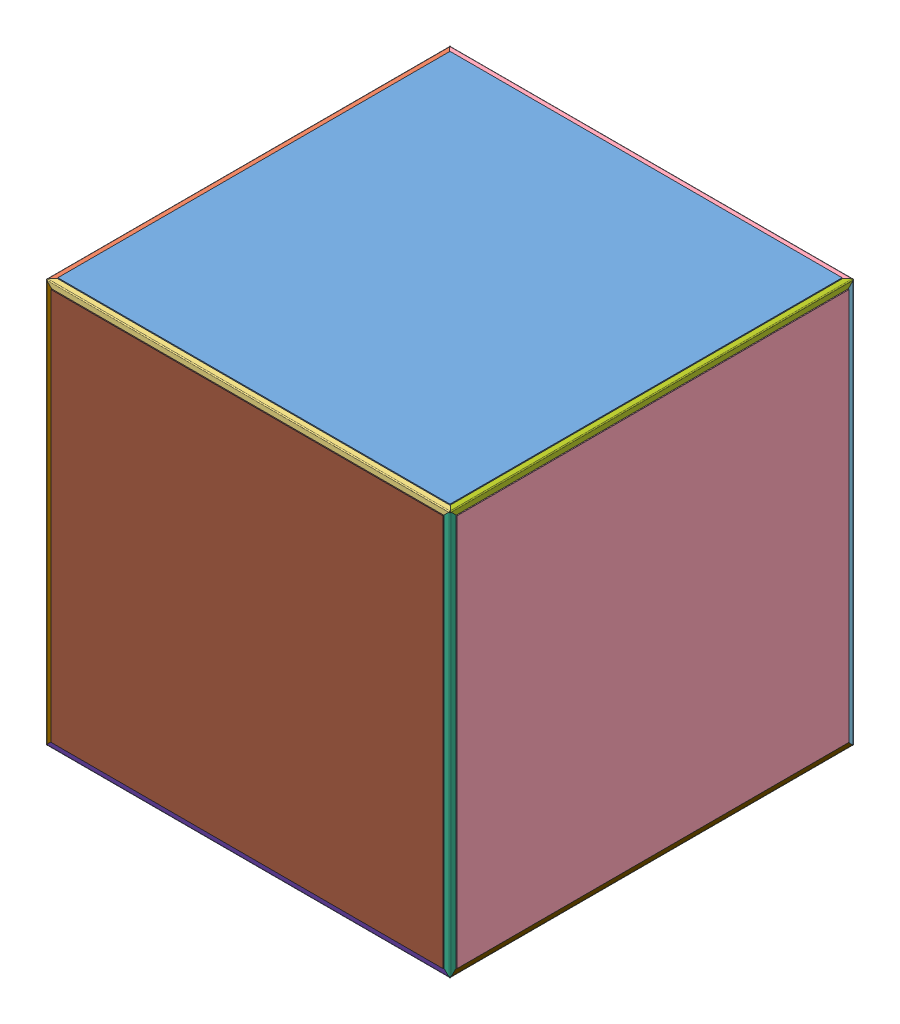
SolidWorks assembly cube_28, configuration cube28. Lengths in mm.
Overall size (661.04 661.04 661.04).
30 component instances, 30 part files, 92 mates.
Components (placement in the parent):
- pr^cube_28-28: pr^cube_28 [cube01] x (-1 0 0) z (0 0 1) size (638.81 1.59 638.81) (virtual)
- dr1^cube_28-55: dr1^cube_28 [cube01] at (-328.3246 328.93 0) x (0 -1 0) z (0 0 1) size (26.01 26.01 657.87) (virtual)
- dr2^cube_28-37: dr2^cube_28 [cube01] at (0 328.93 328.3246) x (0 -1 0) z (1 0 0) size (26.01 26.01 657.87) (virtual)
- dr3^cube_28-33: dr3^cube_28 [cube01] at (0 328.93 -328.3246) x (0 -1 0) z (-1 0 0) size (26.01 26.01 657.87) (virtual)
- br1^cube_28-49: br1^cube_28 [Default] at (0 303.53 -303.53) x (0 0 1) z (-1 0 0) size (50.8 50.8 599.95) (virtual)
- br2^cube_28-61: br2^cube_28 [Default] at (-303.53 303.53 0) size (50.8 50.8 599.95) (virtual)
- br3^cube_28-46: br3^cube_28 [Default] at (0 303.53 303.53) x (0 0 -1) z (1 0 0) size (50.8 50.8 599.95) (virtual)
- pg^cube_28-20: pg^cube_28 [cube01] x (0 -1 0) z (0 0 1) size (638.81 1.59 638.81) (virtual)
- dg1^cube_28-38: dg1^cube_28 [cube01] at (-328.93 0 328.3246) x (1 0 0) z (0 1 0) size (26.01 26.01 657.87) (virtual)
- dg2^cube_28-41: dg2^cube_28 [cube01] at (-328.93 -328.3246 0) size (26.01 26.01 657.87) (virtual)
- dg3^cube_28-34: dg3^cube_28 [cube01] at (-328.93 0 -328.3246) x (1 0 0) z (0 -1 0) size (26.01 26.01 657.87) (virtual)
- bg1^cube_28-47: bg1^cube_28 [Default] at (-303.53 -303.53 0) x (0 1 0) z (0 0 1) size (50.8 50.8 599.95) (virtual)
- bg2^cube_28-44: bg2^cube_28 [Default] at (-303.53 0 303.53) x (0 0 -1) z (0 1 0) size (50.8 50.8 599.95) (virtual)
- bg3^cube_28-40: bg3^cube_28 [Default] at (-303.53 0 -303.53) x (0 0 1) z (0 -1 0) size (50.8 50.8 599.95) (virtual)
- py^cube_28-21: py^cube_28 [cube01] at origin size (638.81 1.59 638.81) (virtual)
- dy1^cube_28-35: dy1^cube_28 [cube01] at (0 -328.93 -328.3246) x (0 1 0) z (1 0 0) size (26.01 26.01 657.87) (virtual)
- dy2^cube_28-39: dy2^cube_28 [cube01] at (0 -328.93 328.3246) x (0 1 0) z (-1 0 0) size (26.01 26.01 657.87) (virtual)
- dy3^cube_28-42: dy3^cube_28 [cube01] at (328.3246 -328.93 0) x (0 1 0) z (0 0 1) size (26.01 26.01 657.87) (virtual)
- by1^cube_28-41: by1^cube_28 [Default] at (0 -303.53 -303.53) x (0 0 1) z (1 0 0) size (50.8 50.8 599.95) (virtual)
- by2^cube_28-45: by2^cube_28 [Default] at (0 -303.53 303.53) x (0 0 -1) z (-1 0 0) size (50.8 50.8 599.95) (virtual)
- by3^cube_28-48: by3^cube_28 [Default] at (303.53 -303.53 0) x (-1 0 0) z (0 0 1) size (50.8 50.8 599.95) (virtual)
- po^cube_28-22: po^cube_28 [cube01] x (0 1 0) z (0 0 1) size (638.81 1.59 638.81) (virtual)
- do1^cube_28-36: do1^cube_28 [cube01] at (328.93 0 -328.3246) x (-1 0 0) z (0 1 0) size (26.01 26.01 657.87) (virtual)
- do2^cube_28-40: do2^cube_28 [cube01] at (328.93 0 328.3246) x (-1 0 0) z (0 -1 0) size (26.01 26.01 657.87) (virtual)
- do3^cube_28-47: do3^cube_28 [cube01] at (328.93 328.3246 0) x (-1 0 0) z (0 0 1) size (26.01 26.01 657.87) (virtual)
- bo1^cube_28-42: bo1^cube_28 [Default] at (303.53 0 -303.53) x (0 0 1) z (0 1 0) size (50.8 50.8 599.95) (virtual)
- bo2^cube_28-46: bo2^cube_28 [Default] at (303.53 0 303.53) x (0 0 -1) z (0 -1 0) size (50.8 50.8 599.95) (virtual)
- bo3^cube_28-62: bo3^cube_28 [Default] at (303.53 303.53 0) x (0 -1 0) z (0 0 1) size (50.8 50.8 599.95) (virtual)
- pc^cube_28-18: pc^cube_28 [cube01] x (-1 0 0) z (0 -1 0) size (638.81 1.59 638.81) (virtual)
- pb^cube_28-21: pb^cube_28 [cube01] x (-1 0 0) z (0 1 0) size (638.81 1.59 638.81) (virtual)
Mates (geometry in assembly coordinates):
- Coincident1: coincident anti-aligned: plane of pr^cube_28-28 through (319.405 328.93 -319.405) normal (0 -1 0); plane of br1^cube_28-49 through (-299.974 328.93 -303.53) normal (0 1 0)
- Coincident2: coincident anti-aligned: plane of pr^cube_28-28 through (319.405 328.93 -319.405) normal (0 -1 0); plane of br2^cube_28-61 through (-303.53 328.93 299.974) normal (0 1 0)
- Coincident3: coincident anti-aligned: plane of pr^cube_28-28 through (319.405 328.93 -319.405) normal (0 -1 0); plane of br3^cube_28-46 through (299.974 328.93 303.53) normal (0 1 0)
- Coincident4: coincident anti-aligned: plane of pr^cube_28-28 through (319.405 328.93 -319.405) normal (0 -1 0); plane of bo3^cube_28-62 through (303.53 328.93 299.974) normal (0 1 0)
- Coincident5: coincident anti-aligned: plane of pr^cube_28-28 through (319.405 328.93 -319.405) normal (0 -1 0); plane of dr3^cube_28-33 through (0 328.93 -657.2546) normal (0 1 0)
- Coincident6: coincident anti-aligned: plane of pr^cube_28-28 through (319.405 328.93 -319.405) normal (0 -1 0); plane of dr1^cube_28-55 through (-657.2546 328.93 0) normal (0 1 0)
- Coincident7: coincident anti-aligned: plane of pr^cube_28-28 through (319.405 328.93 -319.405) normal (0 -1 0); plane of do3^cube_28-47 through (-0.6054 328.93 0) normal (0 1 0)
- Coincident8: coincident anti-aligned: plane of pr^cube_28-28 through (319.405 328.93 -319.405) normal (0 -1 0); plane of dr2^cube_28-37 through (0 328.93 657.2546) normal (0 1 0)
- Coincident34: coincident anti-aligned: plane of pb^cube_28-21 through (319.405 -319.405 -328.93) normal (0 0 1); plane of by1^cube_28-41 through (299.974 -303.53 -328.93) normal (0 0 -1)
- Coincident35: coincident anti-aligned: plane of pb^cube_28-21 through (319.405 -319.405 -328.93) normal (0 0 1); plane of bo1^cube_28-42 through (303.53 299.974 -328.93) normal (0 0 -1)
- Coincident36: coincident anti-aligned: plane of pb^cube_28-21 through (319.405 -319.405 -328.93) normal (0 0 1); plane of br1^cube_28-49 through (-299.974 303.53 -328.93) normal (0 0 -1)
- Coincident37: coincident anti-aligned: plane of pb^cube_28-21 through (319.405 -319.405 -328.93) normal (0 0 1); plane of bg3^cube_28-40 through (-303.53 -299.974 -328.93) normal (0 0 -1)
- Coincident38: coincident anti-aligned: plane of pb^cube_28-21 through (319.405 -319.405 -328.93) normal (0 0 1); plane of dg3^cube_28-34 through (0.6054 0 -328.93) normal (0 0 -1)
- Coincident39: coincident anti-aligned: plane of pb^cube_28-21 through (319.405 -319.405 -328.93) normal (0 0 1); plane of dr3^cube_28-33 through (0 -0.6054 -328.93) normal (0 0 -1)
- Coincident40: coincident anti-aligned: plane of pb^cube_28-21 through (319.405 -319.405 -328.93) normal (0 0 1); plane of do1^cube_28-36 through (-0.6054 0 -328.93) normal (0 0 -1)
- Coincident41: coincident anti-aligned: plane of pb^cube_28-21 through (319.405 -319.405 -328.93) normal (0 0 1); plane of dy1^cube_28-35 through (0 0.6054 -328.93) normal (0 0 -1)
- Coincident42: coincident anti-aligned: plane of pc^cube_28-18 through (319.405 319.405 328.93) normal (0 0 -1); plane of bo2^cube_28-46 through (303.53 -299.974 328.93) normal (0 0 1)
- Coincident43: coincident anti-aligned: plane of pc^cube_28-18 through (319.405 319.405 328.93) normal (0 0 -1); plane of br3^cube_28-46 through (299.974 303.53 328.93) normal (0 0 1)
- Coincident44: coincident anti-aligned: plane of pc^cube_28-18 through (319.405 319.405 328.93) normal (0 0 -1); plane of bg2^cube_28-44 through (-303.53 299.974 328.93) normal (0 0 1)
- Coincident45: coincident anti-aligned: plane of pc^cube_28-18 through (319.405 319.405 328.93) normal (0 0 -1); plane of by2^cube_28-45 through (-299.974 -303.53 328.93) normal (0 0 1)
- Coincident46: coincident anti-aligned: plane of pc^cube_28-18 through (319.405 319.405 328.93) normal (0 0 -1); plane of do2^cube_28-40 through (-0.6054 0 328.93) normal (0 0 1)
- Coincident47: coincident anti-aligned: plane of pc^cube_28-18 through (319.405 319.405 328.93) normal (0 0 -1); plane of dy2^cube_28-39 through (0 0.6054 328.93) normal (0 0 1)
- Coincident48: coincident anti-aligned: plane of pc^cube_28-18 through (319.405 319.405 328.93) normal (0 0 -1); plane of dg1^cube_28-38 through (0.6054 0 328.93) normal (0 0 1)
- Coincident49: coincident anti-aligned: plane of pc^cube_28-18 through (319.405 319.405 328.93) normal (0 0 -1); plane of dr2^cube_28-37 through (0 -0.6054 328.93) normal (0 0 1)
- Coincident50: coincident anti-aligned: plane of pg^cube_28-20 through (-328.93 319.405 -319.405) normal (1 0 0); plane of bg3^cube_28-40 through (-328.93 -299.974 -303.53) normal (-1 0 0)
- Coincident51: coincident anti-aligned: plane of pg^cube_28-20 through (-328.93 319.405 -319.405) normal (1 0 0); plane of bg1^cube_28-47 through (-328.93 -303.53 299.974) normal (-1 0 0)
- Coincident52: coincident anti-aligned: plane of pg^cube_28-20 through (-328.93 319.405 -319.405) normal (1 0 0); plane of bg2^cube_28-44 through (-328.93 299.974 303.53) normal (-1 0 0)
- Coincident53: coincident anti-aligned: plane of pg^cube_28-20 through (-328.93 319.405 -319.405) normal (1 0 0); plane of dr1^cube_28-55 through (-328.93 -0.6054 0) normal (-1 0 0)
- Coincident54: coincident anti-aligned: plane of pg^cube_28-20 through (-328.93 319.405 -319.405) normal (1 0 0); plane of dg3^cube_28-34 through (-328.93 0 -657.2546) normal (-1 0 0)
- Coincident55: coincident anti-aligned: plane of pg^cube_28-20 through (-328.93 319.405 -319.405) normal (1 0 0); plane of dg2^cube_28-41 through (-328.93 -657.2546 0) normal (-1 0 0)
- Coincident56: coincident anti-aligned: plane of pg^cube_28-20 through (-328.93 319.405 -319.405) normal (1 0 0); plane of dg1^cube_28-38 through (-328.93 0 657.2546) normal (-1 0 0)
- Coincident99: coincident anti-aligned: plane of pg^cube_28-20 through (-328.93 319.405 -319.405) normal (1 0 0); plane of br2^cube_28-61 through (-328.93 303.53 299.974) normal (-1 0 0)
- Coincident57: coincident anti-aligned: plane of py^cube_28-21 through (-319.405 -328.93 -319.405) normal (0 1 0); plane of by3^cube_28-48 through (303.53 -328.93 299.974) normal (0 -1 0)
- Coincident58: coincident anti-aligned: plane of py^cube_28-21 through (-319.405 -328.93 -319.405) normal (0 1 0); plane of by2^cube_28-45 through (-299.974 -328.93 303.53) normal (0 -1 0)
- Coincident59: coincident anti-aligned: plane of py^cube_28-21 through (-319.405 -328.93 -319.405) normal (0 1 0); plane of bg1^cube_28-47 through (-303.53 -328.93 299.974) normal (0 -1 0)
- Coincident60: coincident anti-aligned: plane of py^cube_28-21 through (-319.405 -328.93 -319.405) normal (0 1 0); plane of by1^cube_28-41 through (299.974 -328.93 -303.53) normal (0 -1 0)
- Coincident61: coincident anti-aligned: plane of py^cube_28-21 through (-319.405 -328.93 -319.405) normal (0 1 0); plane of dy3^cube_28-42 through (657.2546 -328.93 0) normal (0 -1 0)
- Coincident62: coincident anti-aligned: plane of py^cube_28-21 through (-319.405 -328.93 -319.405) normal (0 1 0); plane of dy2^cube_28-39 through (0 -328.93 657.2546) normal (0 -1 0)
- Coincident63: coincident anti-aligned: plane of py^cube_28-21 through (-319.405 -328.93 -319.405) normal (0 1 0); plane of dg2^cube_28-41 through (0.6054 -328.93 0) normal (0 -1 0)
- Coincident64: coincident anti-aligned: plane of py^cube_28-21 through (-319.405 -328.93 -319.405) normal (0 1 0); plane of dy1^cube_28-35 through (0 -328.93 -657.2546) normal (0 -1 0)
- Coincident65: coincident anti-aligned: plane of po^cube_28-22 through (328.93 -319.405 -319.405) normal (-1 0 0); plane of bo1^cube_28-42 through (328.93 299.974 -303.53) normal (1 0 0)
- Coincident66: coincident anti-aligned: plane of po^cube_28-22 through (328.93 -319.405 -319.405) normal (-1 0 0); plane of by3^cube_28-48 through (328.93 -303.53 299.974) normal (1 0 0)
- Coincident67: coincident anti-aligned: plane of po^cube_28-22 through (328.93 -319.405 -319.405) normal (-1 0 0); plane of bo2^cube_28-46 through (328.93 -299.974 303.53) normal (1 0 0)
- Coincident68: coincident anti-aligned: plane of po^cube_28-22 through (328.93 -319.405 -319.405) normal (-1 0 0); plane of bo3^cube_28-62 through (328.93 303.53 299.974) normal (1 0 0)
- Coincident69: coincident anti-aligned: plane of po^cube_28-22 through (328.93 -319.405 -319.405) normal (-1 0 0); plane of do2^cube_28-40 through (328.93 0 657.2546) normal (1 0 0)
- Coincident70: coincident anti-aligned: plane of po^cube_28-22 through (328.93 -319.405 -319.405) normal (-1 0 0); plane of do3^cube_28-47 through (328.93 657.2546 0) normal (1 0 0)
- Coincident71: coincident anti-aligned: plane of po^cube_28-22 through (328.93 -319.405 -319.405) normal (-1 0 0); plane of do1^cube_28-36 through (328.93 0 -657.2546) normal (1 0 0)
- Coincident72: coincident anti-aligned: plane of po^cube_28-22 through (328.93 -319.405 -319.405) normal (-1 0 0); plane of dy3^cube_28-42 through (328.93 0.6054 0) normal (1 0 0)
- Coincident73: coincident aligned: plane of assembly through (0 0 0) normal (0 0 1); plane of dy3^cube_28-42 through (328.3246 -328.93 0) normal (0 0 1)
- Coincident74: coincident aligned: plane of assembly through (0 0 0) normal (0 0 1); plane of by3^cube_28-48 through (303.53 -303.53 0) normal (0 0 1)
- Coincident75: coincident aligned: plane of assembly through (0 0 0) normal (0 0 1); plane of bo3^cube_28-62 through (303.53 303.53 0) normal (0 0 1)
- Coincident76: coincident aligned: plane of assembly through (0 0 0) normal (0 0 1); plane of do3^cube_28-47 through (328.93 328.3246 0) normal (0 0 1)
- Coincident77: coincident aligned: plane of assembly through (0 0 0) normal (0 0 1); plane of dg2^cube_28-41 through (-328.93 -328.3246 0) normal (0 0 1)
- Coincident78: coincident aligned: plane of assembly through (0 0 0) normal (0 0 1); plane of bg1^cube_28-47 through (-303.53 -303.53 0) normal (0 0 1)
- Coincident79: coincident aligned: plane of assembly through (0 0 0) normal (0 0 1); plane of dr1^cube_28-55 through (-328.3246 328.93 0) normal (0 0 1)
- Coincident80: coincident aligned: plane of assembly through (0 0 0) normal (0 0 1); plane of br2^cube_28-61 through (-303.53 303.53 0) normal (0 0 1)
- Coincident81: coincident aligned: plane of assembly through (0 0 0) normal (0 1 0); plane of bo1^cube_28-42 through (303.53 0 -303.53) normal (0 1 0)
- Coincident82: coincident aligned: plane of assembly through (0 0 0) normal (0 1 0); plane of py^cube_28-21 through (0 0 0) normal (0 1 0)
- Coincident83: coincident aligned: plane of assembly through (0 0 0) normal (0 1 0); plane of do1^cube_28-36 through (328.93 0 -328.3246) normal (0 1 0)
- Coincident84: coincident anti-aligned: plane of assembly through (0 0 0) normal (0 1 0); plane of bg3^cube_28-40 through (-303.53 0 -303.53) normal (0 -1 0)
- Coincident85: coincident anti-aligned: plane of assembly through (0 0 0) normal (0 1 0); plane of dg3^cube_28-34 through (-328.93 0 -328.3246) normal (0 -1 0)
- Coincident86: coincident aligned: plane of assembly through (0 0 0) normal (0 1 0); plane of dg1^cube_28-38 through (-328.93 0 328.3246) normal (0 1 0)
- Coincident87: coincident aligned: plane of assembly through (0 0 0) normal (0 1 0); plane of bg2^cube_28-44 through (-303.53 0 303.53) normal (0 1 0)
- Coincident88: coincident anti-aligned: plane of assembly through (0 0 0) normal (0 1 0); plane of bo2^cube_28-46 through (303.53 0 303.53) normal (0 -1 0)
- Coincident89: coincident anti-aligned: plane of assembly through (0 0 0) normal (0 1 0); plane of do2^cube_28-40 through (328.93 0 328.3246) normal (0 -1 0)
- Coincident90: coincident anti-aligned: plane of assembly through (0 0 0) normal (1 0 0); plane of by2^cube_28-45 through (0 -303.53 303.53) normal (-1 0 0)
- Coincident91: coincident anti-aligned: plane of assembly through (0 0 0) normal (1 0 0); plane of dy2^cube_28-39 through (0 -328.93 328.3246) normal (-1 0 0)
- Coincident92: coincident aligned: plane of assembly through (0 0 0) normal (1 0 0); plane of pg^cube_28-20
- Coincident93: coincident aligned: plane of assembly through (0 0 0) normal (1 0 0); plane of dr2^cube_28-37 through (0 328.93 328.3246) normal (1 0 0)
- Coincident94: coincident aligned: plane of assembly through (0 0 0) normal (1 0 0); plane of br3^cube_28-46 through (0 303.53 303.53) normal (1 0 0)
- Coincident95: coincident anti-aligned: plane of assembly through (0 0 0) normal (1 0 0); plane of dr3^cube_28-33 through (0 328.93 -328.3246) normal (-1 0 0)
- Coincident96: coincident anti-aligned: plane of assembly through (0 0 0) normal (1 0 0); plane of br1^cube_28-49 through (0 303.53 -303.53) normal (-1 0 0)
- Coincident97: coincident aligned: plane of assembly through (0 0 0) normal (1 0 0); plane of by1^cube_28-41 through (0 -303.53 -303.53) normal (1 0 0)
- Coincident98: coincident aligned: plane of assembly through (0 0 0) normal (1 0 0); plane of dy1^cube_28-35 through (0 -328.93 -328.3246) normal (1 0 0)
- Coincident100: coincident anti-aligned: plane of pr^cube_28-28; plane of assembly through (0 0 0) normal (1 0 0)
- Coincident101: coincident aligned: plane of pr^cube_28-28 through (0 0 0) normal (0 0 1); plane of assembly through (0 0 0) normal (0 0 1)
- Coincident102: coincident anti-aligned: plane of pr^cube_28-28; plane of assembly through (0 0 0) normal (0 1 0)
- Coincident106: coincident anti-aligned: plane of pg^cube_28-20; plane of assembly through (0 0 0) normal (0 1 0)
- Coincident107: coincident aligned: plane of pg^cube_28-20; plane of assembly through (0 0 0) normal (1 0 0)
- Coincident108: coincident aligned: plane of pg^cube_28-20 through (0 0 0) normal (0 0 1); plane of assembly through (0 0 0) normal (0 0 1)
- Coincident109: coincident aligned: plane of py^cube_28-21 through (0 0 0) normal (0 0 1); plane of assembly through (0 0 0) normal (0 0 1)
- Coincident110: coincident aligned: plane of py^cube_28-21 through (0 0 0) normal (0 1 0); plane of assembly through (0 0 0) normal (0 1 0)
- Coincident111: coincident aligned: plane of py^cube_28-21 through (0 0 0) normal (1 0 0); plane of assembly through (0 0 0) normal (1 0 0)
- Coincident112: coincident aligned: plane of po^cube_28-22 through (0 0 0) normal (0 0 1); plane of assembly through (0 0 0) normal (0 0 1)
- Coincident113: coincident anti-aligned: plane of po^cube_28-22; plane of assembly through (0 0 0) normal (1 0 0)
- Coincident114: coincident aligned: plane of po^cube_28-22; plane of assembly through (0 0 0) normal (0 1 0)
- Coincident115: coincident anti-aligned: plane of pc^cube_28-18 through (0 0 0) normal (0 -1 0); plane of assembly through (0 0 0) normal (0 1 0)
- Coincident116: coincident anti-aligned: plane of pc^cube_28-18; plane of assembly through (0 0 0) normal (0 0 1)
- Coincident117: coincident anti-aligned: plane of pc^cube_28-18; plane of assembly through (0 0 0) normal (1 0 0)
- Coincident118: coincident aligned: plane of pb^cube_28-21 through (0 0 0) normal (0 1 0); plane of assembly through (0 0 0) normal (0 1 0)
- Coincident119: coincident aligned: plane of pb^cube_28-21; plane of assembly through (0 0 0) normal (0 0 1)
- Coincident120: coincident anti-aligned: line of pb^cube_28-21 through (0.8731 -0.8731 0) axis (0 0 -1); plane of assembly through (0 0 0) normal (1 0 0)
